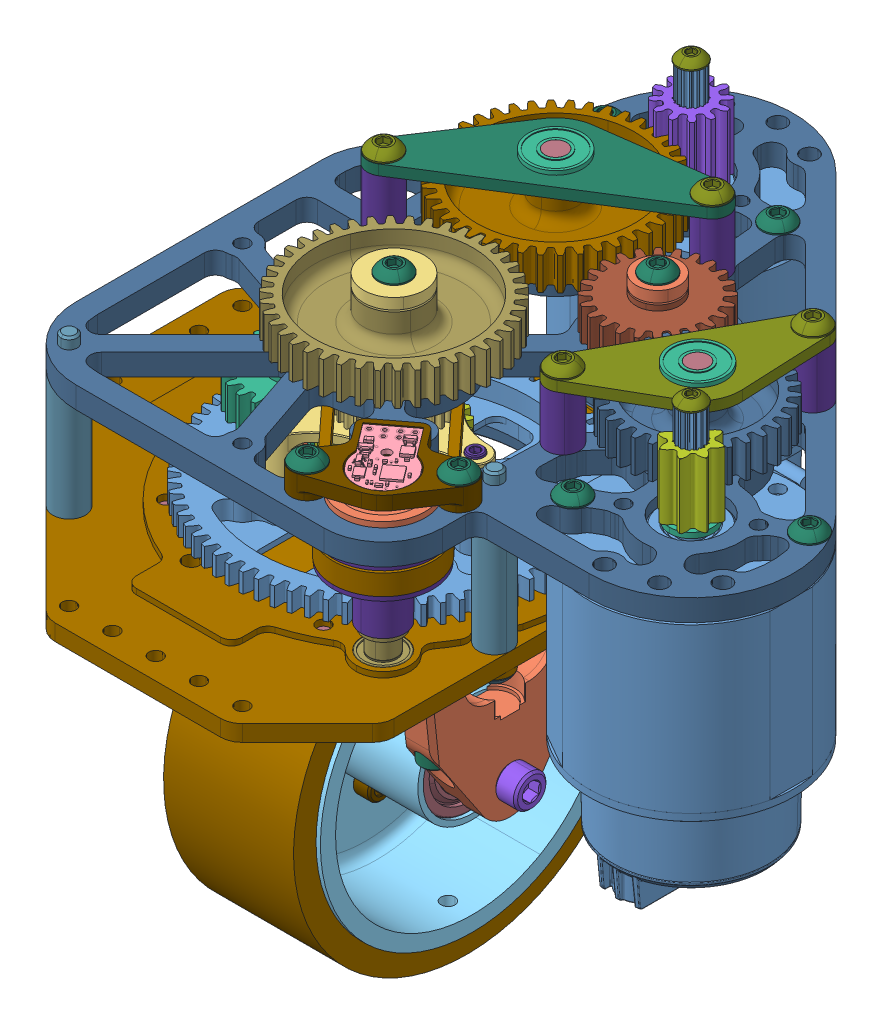
SolidWorks assembly Better Swerve, configuration Default. Lengths in mm.
Overall size (207.33 193.23 207.33).
110 component instances, 63 part files, 0 mates.
Components (placement in the parent):
- WCP-0361 - Swerve X (Tube Mount, Flipped Gears Above).step-1: WCP-0361 - Swerve X (Tube Mount, Flipped Gears Above).step [Default] at origin size (207.33 193.23 207.33)
  - WCP-0364 Rev1 - WCP X Wheel Module.step-1: WCP-0364 Rev1 - WCP X Wheel Module.step [Default] at (0 -0.825 0) size (95.62 174.54 137.74)
    - WCP-0364-001 Rev1.step-1: WCP-0364-001 Rev1.step [Default] at (0 6.35 0) size (93.93 9.53 93.93)
    - WCP-0366 Rev1_Default_As Machined_.step-1: WCP-0366 Rev1_Default_As Machined_.step [Default] at (-29.2862 -49.2125 0) x (0 0 1) z (-1 0 0) size (51.81 60.46 9.5)
    - WCP-0366 Rev1_Default_As Machined_.step-2: WCP-0366 Rev1_Default_As Machined_.step [Default] at (29.2862 -49.2125 0) x (0 0 -1) z (1 0 0) size (51.81 60.46 9.5)
    - WCP-0364-006 Rev1.step-1: WCP-0364-006 Rev1.step [Default] at (0 -49.2125 0) x (1 0 0) z (0 -0.837962 0.545729) size (56.46 12.67 12.67)
    - WCP-0364-005 Rev2.step-1: WCP-0364-005 Rev2.step [Default] at (-29.2862 -1.2827 0) x (0 -1 0) z (0 0 1) size (54.08 11 11)
    - WCP-0365 Rev2.step-1: WCP-0365 Rev2.step [Default] at (2.3061 -49.2125 0) x (0 -0.866025 -0.5) z (1 0 0) size (88.9 88.9 41.15)
    - WCP-0233 Rev1.step-1: WCP-0233 Rev1.step [Default] at (-18.0375 -49.2125 0) x (0 0 -1) z (0 1 0) size (68.52 16.32 68.56)
    - WCP-0364-002 Rev1.step-1: WCP-0364-002 Rev1.step [Default] at (0 34.5757 0) x (0 -1 0) z (0.999257 0 0.03854) size (51.69 15 15)
    - WCP-0276 Rev1.step-1: WCP-0276 Rev1.step [Default] at (-29.2862 -15.4625 0) x (0 0 1) z (1 0 0) size (25.2 12.86 25.34)
    - WCP-0364-008 Rev1.step-1: WCP-0364-008 Rev1.step [Default] at (2.3061 -49.2125 0) x (1 0 0) z (0 -0.879106 0.476626) size (38.1 101.6 101.6)
    - WCP-0357 Rev1.step-1: WCP-0357 Rev1.step [Default] at origin size (88.91 6.35 88.9)
    - WCP-0784_0375_flanged_thunderhex_bearing.step-1: WCP-0784_0375_flanged_thunderhex_bearing.step [Default] at (-29.2862 12.7 0) x (0 -1 0) z (0.06043 0 0.998172) size (7.11 24.61 24.61)
    - WCP-0775_0_250_radial_bearing.step-1: WCP-0775_0_250_radial_bearing.step [Default] at (-29.2862 -29.3687 0) x (0 -1 0) z (0.460874 0 0.887465) size (4.76 12.7 12.7)
    - WCP-0778_0_500_radial_bearing.step-1: WCP-0778_0_500_radial_bearing.step [Default] at (18.0604 -49.2125 0) x (1 0 0) z (0 -0.205758 0.978603) size (7.94 28.57 28.57)
    - WCP-0778_0_500_radial_bearing.step-2: WCP-0778_0_500_radial_bearing.step [Default] at (-17.8424 -49.2125 0) x (1 0 0) z (0 0.040496 0.99918) size (7.94 28.57 28.57)
    - WCP-0781_0_500_flanged_bearing.step-1: WCP-0781_0_500_flanged_bearing.step [Default] at (0 4.7625 0) x (0.999376 0 -0.035335) z (0.035335 0 0.999376) size (31.12 7.94 31.12)
    - NFS-0018_SHCS_#10-32_1_750L_Default_As Machined_.step-1: NFS-0018_SHCS_#10-32_1_750L_Default_As Machined_.step [Default] at (29.2862 11.1125 17.4625) x (0.988526 0 -0.151053) z (0 1 0) size (7.92 7.92 49.28)
    - NFS-0018_SHCS_#10-32_1_750L_Default_As Machined_.step-2: NFS-0018_SHCS_#10-32_1_750L_Default_As Machined_.step [Default] at (29.2862 11.1125 -17.4625) x (0.988526 0 -0.151053) z (0 1 0) size (7.92 7.92 49.28)
    - NFS-0018_SHCS_#10-32_1_750L_Default_As Machined_.step-3: NFS-0018_SHCS_#10-32_1_750L_Default_As Machined_.step [Default] at (-29.2862 11.1125 17.4625) x (0.988526 0 -0.151053) z (0 1 0) size (7.92 7.92 49.28)
    - NFS-0018_SHCS_#10-32_1_750L_Default_As Machined_.step-4: NFS-0018_SHCS_#10-32_1_750L_Default_As Machined_.step [Default] at (-29.2862 11.1125 -17.4625) x (0.988526 0 -0.151053) z (0 1 0) size (7.92 7.92 49.28)
    - 8-32 BHCS_0.500.step-1: 8-32 BHCS_0.500.step [Default] at (-29.2862 23.8633 0) x (0.940105 0 -0.340884) z (0.340884 0 0.940105) size (7.92 14.92 7.92)
    - NFS-0059_SHCS_#4-40_0_875L_91251A113.step-1: NFS-0059_SHCS_#4-40_0_875L_91251A113.step [Default] at (23.876 3.0654 0) x (0.520663 0 0.853762) z (0 -1 0) size (4.65 4.65 25.08)
    - NFS-0059_SHCS_#4-40_0_875L_91251A113.step-2: NFS-0059_SHCS_#4-40_0_875L_91251A113.step [Default] at (-11.938 3.0654 -20.6772) x (0.520663 0 0.853762) z (0 -1 0) size (4.65 4.65 25.08)
    - NFS-0059_SHCS_#4-40_0_875L_91251A113.step-3: NFS-0059_SHCS_#4-40_0_875L_91251A113.step [Default] at (-11.938 3.0654 20.6772) x (0.520663 0 0.853762) z (0 -1 0) size (4.65 4.65 25.08)
    - 10-32 SHCS - No Thread_WCP-0265 - 0.375.step-1: 10-32 SHCS - No Thread_WCP-0265 - 0.375.step [Default] at (-8.2862 -69.85 0) x (0 0.591573 -0.806252) z (0 -0.806252 -0.591573) size (7.67 14.35 7.67)
    - 10-32 SHCS - No Thread_WCP-0265 - 0.375.step-2: 10-32 SHCS - No Thread_WCP-0265 - 0.375.step [Default] at (-8.2862 -38.8937 17.8726) x (0 -0.796051 -0.60523) z (0 -0.60523 0.796051) size (7.67 14.35 7.67)
    - 10-32 SHCS - No Thread_WCP-0265 - 0.375.step-3: 10-32 SHCS - No Thread_WCP-0265 - 0.375.step [Default] at (-8.2862 -59.5312 17.8726) x (0 -0.796051 -0.60523) z (0 -0.60523 0.796051) size (7.67 14.35 7.67)
    - 10-32 SHCS - No Thread_WCP-0265 - 0.375.step-4: 10-32 SHCS - No Thread_WCP-0265 - 0.375.step [Default] at (-8.2862 -59.5312 -17.8726) x (0 -0.796051 -0.60523) z (0 -0.60523 0.796051) size (7.67 14.35 7.67)
    - 10-32 SHCS - No Thread_WCP-0265 - 0.375.step-5: 10-32 SHCS - No Thread_WCP-0265 - 0.375.step [Default] at (-8.2862 -38.8937 -17.8726) x (0 -0.796051 -0.60523) z (0 -0.60523 0.796051) size (7.67 14.35 7.67)
    - 10-32 SHCS - No Thread_WCP-0265 - 0.375.step-6: 10-32 SHCS - No Thread_WCP-0265 - 0.375.step [Default] at (-8.2862 -28.575 0) x (0 -0.796051 -0.60523) z (0 -0.60523 0.796051) size (7.67 14.35 7.67)
    - NFS-0024_250-20_thin_locknut_90566A029.step-1: NFS-0024_250-20_thin_locknut_90566A029.step [Default] at (-34.0362 -49.2125 0) x (0 0.824738 0.565516) z (0 -0.565516 0.824738) size (11.14 5.19 12.86)
    - WCP-0229 Rev1.step-1: WCP-0229 Rev1.step [Default] at (-22.6822 -49.2125 0) size (0.89 16.1 14.34)
    - WCP-0229 Rev1.step-2: WCP-0229 Rev1.step [Default] at (22.6822 -49.2125 0) size (0.89 16.1 14.34)
    - WCP-0367-002 Rev3.step-1: WCP-0367-002 Rev3.step [Default] at (0 28.6559 0) x (0 0 -1) z (1 0 0) size (49.74 26.04 44.2)
    - WCP-0367-006 Rev1.step-1: WCP-0367-006 Rev1.step [Default] at (-29.2862 -3.81 0) size (17.27 17.14 17.27)
    - WCP-0367-010 Rev1.step-1: WCP-0367-010 Rev1.step [Default] at (-29.2862 22.2758 0) x (0 0 1) z (-1 0 0) size (12.7 4.76 12.7)
    - WCP-0434 Rev1.step-1: WCP-0434 Rev1.step [Default] at (-29.2862 19 0) x (-0.327758 0 -0.944762) z (0 -1 0) size (30.3 30.48 12.6)
    - 217-5464_24T_500_hex_steel.step-1: 217-5464_24T_500_hex_steel.step [Default] at (0 19 0) x (0.428371 0 0.903603) z (0 -1 0) size (32.87 32.87 12.6)
    - NFS-0059_SHCS_#4-40_0_875L_91251A113.step-4: NFS-0059_SHCS_#4-40_0_875L_91251A113.step [Default] at (23.876 4.3561 0) x (0.431119 0 0.902295) z (0 -1 0) size (4.65 4.65 25.08)
    - NFS-0059_SHCS_#4-40_0_875L_91251A113.step-5: NFS-0059_SHCS_#4-40_0_875L_91251A113.step [Default] at (-11.938 4.3561 -20.6772) x (0.431119 0 0.902295) z (0 -1 0) size (4.65 4.65 25.08)
    - 0250-20_3L_SHCS_91251A554.step-1: 0250-20_3L_SHCS_91251A554.step [Default] at (-0.8888 -49.2125 0) x (0 -0.133483 -0.991051) z (1 0 0) size (9.53 9.53 82.55)
  - WCP-0360-001 Rev1.step-1: WCP-0360-001 Rev1.step [Default] at origin size (133.35 8 133.35)
  - WCP-0361-001 Rev2.step-1: WCP-0361-001 Rev2.step [Default] at (0 40.4813 0) size (174.12 6.35 174.12)
  - WCP-0364-003 Rev1.step-1: WCP-0364-003 Rev1.step [Default] at (38.669 7.5147 -38.669) x (0.562879 0 0.826539) z (0 1 0) size (20.01 20.32 56.54)
  - WCP-0364-004 Rev1.step-1: WCP-0364-004 Rev1.step [Default] at (36.5633 11.2839 39.7383) x (0 1 0) z (-0.373833 0 -0.927496) size (58.72 11 11)
  - WCP-0361-004 Rev1_Default_As Machined_.step-1: WCP-0361-004 Rev1_Default_As Machined_.step [Default] at (69.0125 51.9621 -19.9819) x (0 1 0) z (0.668276 0 -0.743914) size (25.16 11 11)
  - WCP-0361-004 Rev1_Default_As Machined_.step-2: WCP-0361-004 Rev1_Default_As Machined_.step [Default] at (-5.7166 51.9621 -53.1094) x (0 1 0) z (-0.852362 0 -0.522953) size (25.16 11 11)
  - WCP-0388 Rev1.step-1: WCP-0388 Rev1.step [Default] at (-47.625 19.8438 47.625) x (0 -1 0) z (0.889121 0 -0.457672) size (34.92 9.5 9.5)
  - WCP-0388 Rev1.step-2: WCP-0388 Rev1.step [Default] at (49.2125 19.8438 19.7361) x (0 -1 0) z (0.97467 0 0.223647) size (34.92 9.5 9.5)
  - WCP-0388 Rev1.step-3: WCP-0388 Rev1.step [Default] at (-19.7361 19.8438 -49.2125) x (0 -1 0) z (0.682793 0 0.730612) size (34.92 9.5 9.5)
  - WCP-0361-003 Rev1.step-1: WCP-0361-003 Rev1.step [Default] at (-5.7166 61.0312 -53.1094) x (0.846103 0 -0.533019) z (0.533019 0 0.846103) size (79.38 3 24.61)
  - WCP-0361-006 Rev1.step-1: WCP-0361-006 Rev1.step [Default] at (69.0125 61.0312 -19.9819) x (0.481501 0 -0.876446) z (0.876446 0 0.481501) size (63.5 3 24.61)
  - WCP-0203 Rev1.step-1: WCP-0203 Rev1.step [Default] at (49.7569 51.5938 0.2314) x (0 -1 0) z (-0.759691 0 -0.650284) size (15.88 9.5 9.5)
  - WCP-0203 Rev1.step-2: WCP-0203 Rev1.step [Default] at (75.7459 51.5938 -47.0747) x (0 -1 0) z (0.825334 0 0.564645) size (15.88 9.5 9.5)
  - WCP-0203 Rev1.step-3: WCP-0203 Rev1.step [Default] at (27.6413 51.5938 -65.6808) x (0 -1 0) z (-0.22935 0 -0.973344) size (15.88 9.5 9.5)
  - WCP-0203 Rev1.step-4: WCP-0203 Rev1.step [Default] at (-31.459 51.5938 -28.4494) x (0 -1 0) z (0.432553 0 -0.901608) size (15.88 9.5 9.5)
  - WCP-0307 Rev1.step-1: WCP-0307 Rev1.step [Default] at (-19.7361 -5.5913 -49.2125) x (0 -1 0) z (0.829544 0 0.558441) size (3.18 9.5 9.5)
  - 217-6515_Falcon_500_Default_As Machined_.step-1: 217-6515_Falcon_500_Default_As Machined_.step [Default] at (0.16 11.1062 -86.9695) x (0.5 0 0.866025) z (0 1 0) size (60 60 115.81)
  - 217-6515_Falcon_500_Default_As Machined_.step-2: 217-6515_Falcon_500_Default_As Machined_.step [Default] at (86.9695 11.1062 -0.16) x (0.866025 0 -0.5) z (0 1 0) size (60 60 115.81)
  - WCP-0779_0_375_flanged_bearing.step-1: WCP-0779_0_375_flanged_bearing.step [Default] at (36.5633 45.2437 39.7383) x (0 -1 0) z (0.710471 0 -0.703726) size (7.11 24.61 24.61)
  - WCP-0775_0_250_radial_bearing.step-1: WCP-0775_0_250_radial_bearing.step [Default] at (36.5633 1.6187 39.7383) x (0 1 0) z (-0.269707 0 0.962942) size (4.76 12.7 12.7)
  - WCP-0041_0_250_radial_bearing.step-1: WCP-0041_0_250_radial_bearing.step [Default] at (38.669 1.5108 -38.669) x (-0.316483 0 0.948598) z (0 -1 0) size (15.88 15.88 4.98)
  - WCP-0785_0_500_flanged_thunderhex_bearing.step-1: WCP-0785_0_500_flanged_thunderhex_bearing.step [Default] at (0 39.6875 0) x (-0.903668 0 0.428233) z (0 -1 0) size (31.12 31.12 7.94)
  - 217-2735_0_375_flanged_hex_bearing.step-1: 217-2735_0_375_flanged_hex_bearing.step [Default] at (38.669 43.6562 -38.669) x (0.628897 0 0.777488) z (0.777488 0 -0.628897) size (31.12 7.94 31.12)
  - WCP-0779_0_375_flanged_bearing.step-2: WCP-0779_0_375_flanged_bearing.step [Default] at (69.0125 45.2437 -19.9819) x (0 -1 0) z (-0.896651 0 -0.442737) size (7.11 24.61 24.61)
  - WCP-0779_0_375_flanged_bearing.step-3: WCP-0779_0_375_flanged_bearing.step [Default] at (-5.7166 45.2437 -53.1094) x (0 -1 0) z (0.589783 0 0.807562) size (7.11 24.61 24.61)
  - WCP-0042_0_250_flanged_bearing.step-1: WCP-0042_0_250_flanged_bearing.step [Default] at (69.0125 61.2077 -19.9819) x (0.808515 0 -0.588476) z (0 -1 0) size (18.24 18.24 4.98)
  - WCP-0042_0_250_flanged_bearing.step-2: WCP-0042_0_250_flanged_bearing.step [Default] at (-5.7166 61.2077 -53.1094) x (0.808515 0 -0.588476) z (0 -1 0) size (18.24 18.24 4.98)
  - 217-6915_Falcon_8T.step-1: 217-6915_Falcon_8T.step [Default] at (86.9695 53.0588 -0.16) x (0.660796 0 -0.750566) z (0 -1 0) size (13.62 13.62 19.06)
  - 217-6919_Falcon_12T.step-1: 217-6919_Falcon_12T.step [Default] at (0.16 53.0588 -86.9695) x (-0.693192 0 0.720753) z (0 1 0) size (17.78 17.78 19.05)
  - WCP-0541 Rev1.step-1: WCP-0541 Rev1.step [Default] at (-5.7166 51.5684 -53.1094) x (0.292927 0 0.956135) z (0 1 0) size (55.8 55.88 12.65)
  - WCP-0540 Rev1.step-1: WCP-0540 Rev1.step [Default] at (69.0125 51.5438 -19.9819) x (0.820194 0 -0.572086) z (0 1 0) size (43.07 43.07 12.6)
  - WCP-0538 Rev1.step-1: WCP-0538 Rev1.step [Default] at (38.669 51.5684 -38.669) x (0.37732 0 0.926083) z (0 -1 0) size (32.86 32.86 12.65)
  - WCP-0178 Rev1.step-1: WCP-0178 Rev1.step [Default] at (0 51.5684 0) x (0.927258 0 0.374423) z (0 1 0) size (55.8 55.88 12.65)
  - 10-32 BHCS - No Thread_WCP-0251 - 0.250.step-1: 10-32 BHCS - No Thread_WCP-0251 - 0.250.step [Default] at (-33.4155 -4 33.4155) x (0.140263 0 -0.990114) z (-0.990114 0 -0.140263) size (9.17 8.92 9.17)
  - 10-32 BHCS - No Thread_WCP-0259 - 2.000.step-1: 10-32 BHCS - No Thread_WCP-0259 - 2.000.step [Default] at (-47.625 -4 47.625) x (0.999892 0 -0.01471) z (-0.01471 0 -0.999892) size (9.17 53.37 9.17)
  - 10-32 BHCS - No Thread_WCP-0259 - 2.000.step-2: 10-32 BHCS - No Thread_WCP-0259 - 2.000.step [Default] at (49.2125 -4 19.7361) x (0.334009 0 -0.94257) z (-0.94257 0 -0.334009) size (9.17 53.37 9.17)
  - 10-32 BHCS - No Thread_WCP-0259 - 2.000.step-3: 10-32 BHCS - No Thread_WCP-0259 - 2.000.step [Default] at (-19.7361 -7.175 -49.2125) x (-0.998904 0 -0.046801) z (-0.046801 0 0.998904) size (9.17 53.37 9.17)
  - 10-32 BHCS - No Thread_WCP-0253 - 0.500.step-1: 10-32 BHCS - No Thread_WCP-0253 - 0.500.step [Default] at (23.914 50.2348 49.3306) x (-0.169382 0 -0.98555) z (0.98555 0 -0.169382) size (9.17 15.27 9.17)
  - 10-32 BHCS - No Thread_WCP-0253 - 0.500.step-2: 10-32 BHCS - No Thread_WCP-0253 - 0.500.step [Default] at (49.2125 50.2348 30.146) x (0.162273 0 -0.986746) z (0.986746 0 0.162273) size (9.17 15.27 9.17)
  - 8-32 BHCS_0.500.step-1: 8-32 BHCS_0.500.step [Default] at (86.9695 72.1088 -0.16) x (-0.999431 0 -0.033743) z (0.033743 0 -0.999431) size (7.92 14.92 7.92)
  - 8-32 BHCS_0.500.step-2: 8-32 BHCS_0.500.step [Default] at (0.16 72.1088 -86.9695) x (0.994914 0 -0.100726) z (0.100726 0 0.994914) size (7.92 14.92 7.92)
  - 10-32 BHCS - No Thread_WCP-0255 - 1.000.step-1: 10-32 BHCS - No Thread_WCP-0255 - 1.000.step [Default] at (-31.459 62.5312 -28.4494) x (0.932842 0 -0.360285) z (0.360285 0 0.932842) size (9.17 27.97 9.17)
  - 10-32 BHCS - No Thread_WCP-0255 - 1.000.step-2: 10-32 BHCS - No Thread_WCP-0255 - 1.000.step [Default] at (75.7459 62.5312 -47.0747) x (-0.965073 0 0.261981) z (-0.261981 0 -0.965073) size (9.17 27.97 9.17)
  - 10-32 BHCS - No Thread_WCP-0255 - 1.000.step-3: 10-32 BHCS - No Thread_WCP-0255 - 1.000.step [Default] at (49.7569 62.5312 0.2314) x (0.400913 0 0.916116) z (-0.916116 0 0.400913) size (9.17 27.97 9.17)
  - 10-32 BHCS - No Thread_WCP-0255 - 1.000.step-4: 10-32 BHCS - No Thread_WCP-0255 - 1.000.step [Default] at (27.6413 62.5312 -65.6808) x (0.279232 0 -0.960224) z (0.960224 0 0.279232) size (9.17 27.97 9.17)
  - 10-32 BHCS - No Thread_WCP-0253 - 0.500.step-3: 10-32 BHCS - No Thread_WCP-0253 - 0.500.step [Default] at (64.9724 43.6562 12.54) x (-0.441083 0 0.897466) z (-0.897466 0 -0.441083) size (9.17 15.27 9.17)
  - 10-32 BHCS - No Thread_WCP-0253 - 0.500.step-4: 10-32 BHCS - No Thread_WCP-0253 - 0.500.step [Default] at (108.9665 43.6562 -12.86) x (-0.441083 0 0.897466) z (-0.897466 0 -0.441083) size (9.17 15.27 9.17)
  - 10-32 BHCS - No Thread_WCP-0253 - 0.500.step-5: 10-32 BHCS - No Thread_WCP-0253 - 0.500.step [Default] at (-25.24 43.6562 -86.9695) x (-0.441083 0 0.897466) z (-0.897466 0 -0.441083) size (9.17 15.27 9.17)
  - 10-32 BHCS - No Thread_WCP-0253 - 0.500.step-6: 10-32 BHCS - No Thread_WCP-0253 - 0.500.step [Default] at (25.56 43.6562 -86.9695) x (-0.441083 0 0.897466) z (-0.897466 0 -0.441083) size (9.17 15.27 9.17)
  - 10-32 BHCS - No Thread_WCP-0253 - 0.500.step-7: 10-32 BHCS - No Thread_WCP-0253 - 0.500.step [Default] at (38.669 61.5691 -38.669) x (0.905057 0 -0.425291) z (0.425291 0 0.905057) size (9.17 15.27 9.17)
  - 10-32 BHCS - No Thread_WCP-0253 - 0.500.step-8: 10-32 BHCS - No Thread_WCP-0253 - 0.500.step [Default] at (0 61.5828 0) x (0.486688 0 -0.873576) z (0.873576 0 0.486688) size (9.17 15.27 9.17)
  - WCP-0367-003 Rev2.step-1: WCP-0367-003 Rev2.step [Default] at (36.5633 36.3309 39.7383) x (0.013698 0 -0.999906) z (0 1 0) size (29.05 29.05 26.83)
  - WCP-0367-012 Rev1_Straight.step-1: WCP-0367-012 Rev1_Straight.step [Default] at (36.5633 48.2156 39.7383) x (-0.796803 0 0.604239) z (-0.604239 0 -0.796803) size (41.27 6.58 26.97)
  - WCP-0367-001 Rev1.step-1: WCP-0367-001 Rev1.step [Default] at (0 35.3446 0) x (0.996516 0 -0.083401) z (0.083401 0 0.996516) size (19.05 0.51 19.05)
  - WCP-0367-014 Rev1.step-1: WCP-0367-014 Rev1.step [Default] at (38.669 58.3941 -38.669) x (0.434364 0 -0.900737) z (-0.900737 0 -0.434364) size (12.7 6.01 12.7)
  - WCP-0367-013 Rev1.step-1: WCP-0367-013 Rev1.step [Default] at (0 58.4078 0) x (-0.533005 0 0.846112) z (0.846112 0 0.533005) size (17.78 5.96 17.78)
  - 10-32 BHCS - No Thread_WCP-0251 - 0.250.step-2: 10-32 BHCS - No Thread_WCP-0251 - 0.250.step [Default] at (-42.106 -4 -21.4541) x (0.984998 0 -0.172564) z (-0.172564 0 -0.984998) size (9.17 8.92 9.17)
  - 10-32 BHCS - No Thread_WCP-0251 - 0.250.step-3: 10-32 BHCS - No Thread_WCP-0251 - 0.250.step [Default] at (7.3926 -4 -46.6749) x (0.4685 0 0.883464) z (0.883464 0 -0.4685) size (9.17 8.92 9.17)
  - 10-32 BHCS - No Thread_WCP-0251 - 0.250.step-4: 10-32 BHCS - No Thread_WCP-0251 - 0.250.step [Default] at (46.6749 -4 -7.3926) x (-0.69545 0 0.718575) z (0.718575 0 0.69545) size (9.17 8.92 9.17)
  - 10-32 BHCS - No Thread_WCP-0251 - 0.250.step-5: 10-32 BHCS - No Thread_WCP-0251 - 0.250.step [Default] at (21.4541 -4 42.106) x (-0.898311 0 -0.43936) z (-0.43936 0 0.898311) size (9.17 8.92 9.17)
  - CANcoder.step-1: CANcoder.step [Default] at (36.5426 46.4546 39.732) x (-0.796803 0 0.604239) z (0 1 0) size (15.94 23.28 4.54)
  - WCP-0156 Rev1.step-1: WCP-0156 Rev1.step [Default] at (36.5633 38.8937 39.7383) size (6.35 12.7 6.35)
  - Falcon_Motor_Spacer_0625.step-1: Falcon_Motor_Spacer_0625.step [Default] at (86.9695 42.74 -0.16) size (12.7 1.59 12.7)
  - Falcon_Motor_Spacer_0625.step-2: Falcon_Motor_Spacer_0625.step [Default] at (0.16 42.74 -86.9695) x (0.98238 0 0.186896) z (-0.186896 0 0.98238) size (12.7 1.59 12.7)
  - WCP-0787_0625L_500_hex.step-1: WCP-0787_0625L_500_hex.step [Default] at (0 44.45 0) x (0.567835 0 0.823143) z (0 -1 0) size (19.5 19.5 1.59)
  - 217-3258_0625L_375_hex.step-1: 217-3258_0625L_375_hex.step [Default] at (38.669 44.45 -38.669) x (0.988675 0 0.150072) z (0 1 0) size (15.88 15.88 1.59)
  - Encoder Belt.step-1: Encoder Belt.step [Default] at (18.2816 30.8309 19.8691) x (0.677097 0 0.735894) z (-0.735894 0 0.677097) size (83.28 6 29.28)
